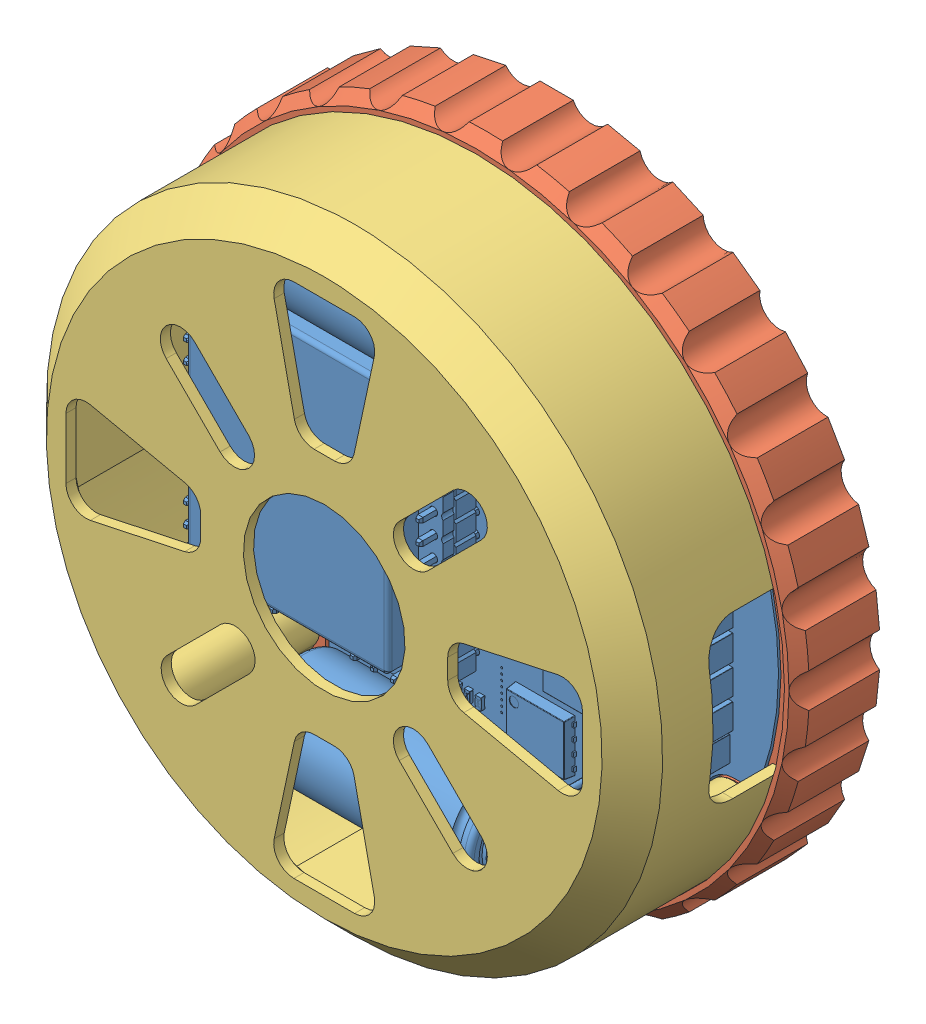
SolidWorks assembly openmyxa_enclosure, configuration Default. Lengths in mm.
Overall size (64.31 64.31 28).
20 component instances, 11 part files, 19 mates.
Components (placement in the parent):
- OpenMyxa-1: OpenMyxa [Default] at origin size (57.99 58 20.52)
- bottom_enclosure-1: bottom_enclosure [Default] at origin size (64.31 64.31 8)
- top_enclosure-1: top_enclosure [Default] at (0 0 1.6) x (0 1 0) z (0 0 1) size (61 61 16)
- cover-2: cover [Default] at (-0.023 0 -5.4) x (1 0 0) z (0 0 -1) size (59.82 30.31 5)
- socket head cap screw_din-6: socket head cap screw_din [DIN 912 M2 x 4 --- 4S] at (26.1493 0 -8.4) x (0 0 1) z (-1 0 0) size (6 3.8 3.8)
- socket head cap screw_din-7: socket head cap screw_din [DIN 912 M2 x 4 --- 4S] at (-27.023 11.8 -8.4) x (0 0 1) z (-1 0 0) size (6 3.8 3.8)
- socket head cap screw_din-8: socket head cap screw_din [DIN 912 M2 x 4 --- 4S] at (-27.063 -11.8 -8.4) x (0 0 1) z (-1 0 0) size (6 3.8 3.8)
- ASM000_TMOTOR_U8-1: ASM000_TMOTOR_U8 [Default] at (0 0 44.1) x (0.030947 -0.999521 0) z (-0.999521 -0.030947 0) size (88.66 26.69 87.17) (hidden)
  - 020_U8_STATOR_HOUSING-1: 020_U8_STATOR_HOUSING [Default] at origin size (86.8 18.69 86.8)
  - 010_U8_ROTOR-1: 010_U8_ROTOR [Default] at origin size (88.66 24.5 87.17)
  - 021_U8_STATOR_COILS-1: 021_U8_STATOR_COILS [Default] at (0 -12.5 0) size (81 11.5 81)
  - 5972K155_BALL BEARING-1: 5972K155_BALL BEARING [5972K155] at (0 -10.5 0) x (1 0 0) z (0 -1 0) size (24 24 5)
  - 5972K155_BALL BEARING-2: 5972K155_BALL BEARING [5972K155] at (0 -22 0) x (1 0 0) z (0 -1 0) size (24 24 5)
  - 011_U8_ROTOR_CAP-1: 011_U8_ROTOR_CAP [Default] at (0 -24.5 0) x (1 0 0) z (0 0 -1) size (18.5 2 18.5)
  - 91294A128_BLACK ALLOY STEEL FLAT-HEAD SOCKET CAP SCREW-1: 91294A128_BLACK ALLOY STEEL FLAT-HEAD SOCKET CAP SCREW [91294A128] at (0 -26.5 5.5) x (1 0 0) z (0 -1 0) size (6 6 8.29)
  - 91294A128_BLACK ALLOY STEEL FLAT-HEAD SOCKET CAP SCREW-2: 91294A128_BLACK ALLOY STEEL FLAT-HEAD SOCKET CAP SCREW [91294A128] at (0 -26.5 -5.5) x (0.999066 0 -0.043219) z (0 -1 0) size (6 6 8.29)
- socket head cap screw_din-17: socket head cap screw_din [DIN 912 M3 x 16 --- 16S] at (-19 -19 -4.9) x (0 0 1) z (-1 0 0) size (19 5.5 5.5)
- socket head cap screw_din-18: socket head cap screw_din [DIN 912 M3 x 16 --- 16S] at (24.4 14 -4.9) x (0 0 1) z (-1 0 0) size (19 5.5 5.5)
- socket head cap screw_din-19: socket head cap screw_din [DIN 912 M3 x 16 --- 16S] at (24.4 -14 -4.9) x (0 0 1) z (-1 0 0) size (19 5.5 5.5)
- socket head cap screw_din-20: socket head cap screw_din [DIN 912 M3 x 16 --- 16S] at (-19 19 -4.9) x (0 0 1) z (-1 0 0) size (19 5.5 5.5)
Mates (geometry in assembly coordinates):
- Coincident6: coincident anti-aligned: plane of bottom_enclosure-1 through (0 0 1.6) normal (0 0 1); plane of top_enclosure-1 through (0 0 1.6) normal (0 0 -1)
- Угол1: planar angle = 3.141593 rad aligned: plane of top_enclosure-1 through (0 0 1.6) normal (-1 0 0); plane of bottom_enclosure-1 through (0 0 0) normal (1 0 0)
- Совпадение14: coincident anti-aligned: plane of bottom_enclosure-1 through (0 0 -5.4) normal (0 0 -1); plane of cover-2 through (-1.3337 13 -5.4) normal (0 0 1)
- Совпадение22: coincident anti-aligned: plane of cover-2 through (0 0 -6.4) normal (0 0 -1); plane of socket head cap screw_din-8 through (-27.063 -9.9 -6.4) normal (0 0 1)
- Концентричный8: concentric aligned: circle of cover-2; circle of socket head cap screw_din-8
- Концентричный9: concentric anti-aligned: circle of cover-2; circle of socket head cap screw_din-7
- Совпадение23: coincident anti-aligned: plane of cover-2 through (0 0 -6.4) normal (0 0 -1); plane of socket head cap screw_din-7 through (-27.023 13.7 -6.4) normal (0 0 1)
- Совпадение24: coincident anti-aligned: plane of cover-2 through (26.1493 0 -6.4) normal (0 0 -1); plane of socket head cap screw_din-6 through (26.1493 1.9 -6.4) normal (0 0 1)
- Концентричный10: concentric aligned: circle of cover-2; circle of socket head cap screw_din-6
- Концентричный13: concentric anti-aligned: circle of top_enclosure-1; circle of ASM000_TMOTOR_U8-1/011_U8_ROTOR_CAP-1
- Совпадение27: coincident anti-aligned: plane of top_enclosure-1 through (0 0 17.6) normal (0 0 1); plane of ASM000_TMOTOR_U8-1/020_U8_STATOR_HOUSING-1 through (0.3714 -11.9943 17.6) normal (0 0 -1)
- Совпадение35: coincident anti-aligned: plane of bottom_enclosure-1 through (24.4 -14 -1.9) normal (0 0 -1); plane of socket head cap screw_din-17 through (-19 -16.25 -1.9) normal (0 0 1)
- Концентричный21: concentric anti-aligned: circle of bottom_enclosure-1; circle of socket head cap screw_din-17
- Совпадение36: coincident anti-aligned: plane of bottom_enclosure-1 through (24.4 -14 -1.9) normal (0 0 -1); plane of socket head cap screw_din-20 through (-19 21.75 -1.9) normal (0 0 1)
- Совпадение37: coincident anti-aligned: plane of bottom_enclosure-1 through (24.4 14 -1.9) normal (0 0 -1); plane of socket head cap screw_din-19 through (24.4 -11.25 -1.9) normal (0 0 1)
- Совпадение38: coincident anti-aligned: plane of bottom_enclosure-1 through (-19 19 -1.9) normal (0 0 -1); plane of socket head cap screw_din-18 through (24.4 16.75 -1.9) normal (0 0 1)
- Концентричный22: concentric anti-aligned: circle of bottom_enclosure-1; circle of socket head cap screw_din-18
- Концентричный23: concentric aligned: circle of bottom_enclosure-1; circle of socket head cap screw_din-19
- Концентричный24: concentric anti-aligned: circle of bottom_enclosure-1; circle of socket head cap screw_din-20
